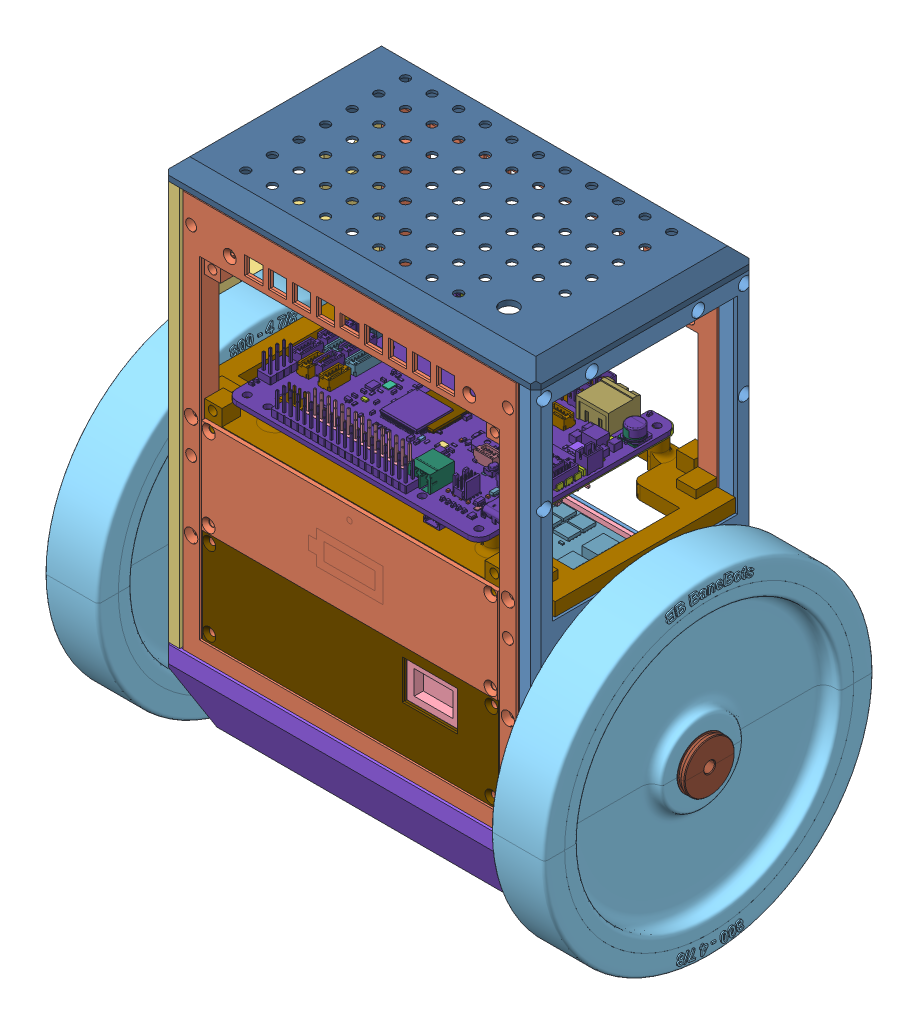
SolidWorks assembly twipr_v2, configuration Default. Lengths in mm.
Overall size (189.01 198.92 123.83).
484 component instances, 75 part files, 68 mates.
Components (placement in the parent):
- twipr_sketch-1: twipr_sketch [Default] at origin size (188 200.75 0) (hidden)
- brace_right-2: brace_right [Default] at (-379.6774 202.2203 0) x (0 0 -1) z (1 0 0) size (82 150 7)
- brace_front_led-1: brace_front_led [Default] at (-442.6774 202.2203 -41) size (126 150 7)
- brace_left_display-2: brace_left_display [Default] at (-505.6774 202.2203 0) x (0 0 1) z (-1 0 0) size (82 150 8)
- brace_front_led-2: brace_front_led [Default] at (-442.6774 202.2203 41) x (-1 0 0) z (0 0 -1) size (126 150 7)
- platform_middle_big_bms-1: platform_middle_big_bms [Default] at (-442.7274 165.7203 0) size (126 42 78.8)
- banebots_4_78-1: banebots_4_78 [Default] at (-368.872 147.2203 0) x (0 0 -1) z (1 0 0) size (123.83 123.83 21.34)
- banebots_4_78-2: banebots_4_78 [Default] at (-516.2261 147.2203 0) x (0 0 1) z (-1 0 0) size (123.83 123.83 21.34)
- robot-hub-1: robot-hub [Default] at (-323.8774 212.8203 108.5) x (-1 0 0) z (0 1 0) size (91.46 70 13.31)
  - robot-hub.step-1: robot-hub.step [Default] at origin size (91.46 70 13.31)
    - R_0603_1608Metric.step-1: R_0603_1608Metric.step [Default] at (112.6 -91.1 1.71) x (0 1 0) z (0 0 1) size (1.6 0.8 0.45)
      - SOLID.step-1: SOLID.step [Default] at origin size (1.6 0.8 0.45)
    - C_1210_3225Metric.step-1: C_1210_3225Metric.step [Default] at (76.55 -102.85 1.71) x (-1 0 0) z (0 0 1) size (3.2 2.5 2.5)
      - SOLID-0.step-1: SOLID-0.step [Default] at origin size (3.2 2.5 2.5)
    - C_0603_1608Metric.step-1: C_0603_1608Metric.step [Default] at (132.2 -95.8 1.71) x (0 1 0) z (0 0 1) size (1.6 0.8 0.8)
      - SOLID-1.step-1: SOLID-1.step [Default] at origin size (1.6 0.8 0.8)
    - JST_GH_BM04B-GHS-TBT_1x04-1MP_P1.25mm_Vertical.step-1: JST_GH_BM04B-GHS-TBT_1x04-1MP_P1.25mm_Vertical.step [Default] at (152.6 -95.3 1.71) x (0 1 0) z (0 0 1) size (8.25 4.95 4.2)
      - SOLID-2.step-1: SOLID-2.step [Default] at origin size (8.25 4.95 4.2)
    - R_0603_1608Metric.step-2: R_0603_1608Metric.step [Default] at (107.5 -84.7687 1.71) x (0 -1 0) z (0 0 1) size (1.6 0.8 0.45)
      - SOLID.step-1: SOLID.step [Default] at origin size (1.6 0.8 0.45)
    - R_0402_1005Metric.step-1: R_0402_1005Metric.step [Default] at (123.5 -93.2 1.71) x (0 1 0) z (0 0 1) size (1 0.5 0.35)
      - SOLID-3.step-1: SOLID-3.step [Default] at origin size (1 0.5 0.35)
    - LED_0603_1608Metric.step-1: LED_0603_1608Metric.step [Default] at (88 -81.3 1.71) x (0 -1 0) z (0 0 1) size (1.6 0.8 1.1)
      - SOLID-4.step-1: SOLID-4.step [Default] at origin size (1.6 0.8 1.1)
    - R_0603_1608Metric.step-3: R_0603_1608Metric.step [Default] at (113.4 -101.6 1.71) x (-1 0 0) z (0 0 1) size (1.6 0.8 0.45)
      - SOLID.step-1: SOLID.step [Default] at origin size (1.6 0.8 0.45)
    - LTC4412ES6#TRMPBF.step-1: LTC4412ES6#TRMPBF.step [Default] at (86.1 -94.6 1.71) size (2.8 2.9 1)
      - COMPOUND.step-1: COMPOUND.step [Default] at origin size (2.8 2.9 1)
    - ws2812_2020.step-1: ws2812_2020.step [Default] at (84.3 -81.3 1.71) size (2.2 2 0.84)
      - COMPOUND-5.step-1: COMPOUND-5.step [Default] at origin size (2.2 2 0.84)
    - LED_0603_1608Metric.step-2: LED_0603_1608Metric.step [Default] at (86.1 -86.8 1.71) size (1.6 0.8 1.1)
      - SOLID-4.step-1: SOLID-4.step [Default] at origin size (1.6 0.8 1.1)
    - R_0402_1005Metric.step-2: R_0402_1005Metric.step [Default] at (133.8 -92.9 1.71) x (0 -1 0) z (0 0 1) size (1 0.5 0.35)
      - SOLID-3.step-1: SOLID-3.step [Default] at origin size (1 0.5 0.35)
    - JST_GH_BM06B-GHS-TBT_1x06-1MP_P1.25mm_Vertical.step-1: JST_GH_BM06B-GHS-TBT_1x06-1MP_P1.25mm_Vertical.step [Default] at (114 -135.2 1.71) size (10.75 4.95 4.2)
      - SOLID-6.step-1: SOLID-6.step [Default] at origin size (10.75 4.95 4.2)
    - JST_GH_BM04B-GHS-TBT_1x04-1MP_P1.25mm_Vertical.step-2: JST_GH_BM04B-GHS-TBT_1x04-1MP_P1.25mm_Vertical.step [Default] at (134.6 -135.2 1.71) size (8.25 4.95 4.2)
      - SOLID-2.step-1: SOLID-2.step [Default] at origin size (8.25 4.95 4.2)
    - C_0603_1608Metric.step-2: C_0603_1608Metric.step [Default] at (109.4 -97.4 1.71) x (-1 0 0) z (0 0 1) size (1.6 0.8 0.8)
      - SOLID-1.step-1: SOLID-1.step [Default] at origin size (1.6 0.8 0.8)
    - C_1210_3225Metric.step-2: C_1210_3225Metric.step [Default] at (87.55 -126.8 1.71) size (3.2 2.5 2.5)
      - SOLID-0.step-1: SOLID-0.step [Default] at origin size (3.2 2.5 2.5)
    - C_1210_3225Metric.step-3: C_1210_3225Metric.step [Default] at (76.55 -109.6 1.71) x (-1 0 0) z (0 0 1) size (3.2 2.5 2.5)
      - SOLID-0.step-1: SOLID-0.step [Default] at origin size (3.2 2.5 2.5)
    - R_0603_1608Metric.step-4: R_0603_1608Metric.step [Default] at (138.6 -95.5 1.71) x (0 -1 0) z (0 0 1) size (1.6 0.8 0.45)
      - SOLID.step-1: SOLID.step [Default] at origin size (1.6 0.8 0.45)
    - CP_Elec_6.3x5.2.step-1: CP_Elec_6.3x5.2.step [Default] at (77.8 -133.7 1.71) x (0 1 0) z (0 0 1) size (10.2 10.92 5.2)
      - SOLID-7.step-1: SOLID-7.step [Default] at origin size (10.2 10.92 5.2)
    - R_0402_1005Metric.step-3: R_0402_1005Metric.step [Default] at (127.9 -91.7 1.71) x (0 -1 0) z (0 0 1) size (1 0.5 0.35)
      - SOLID-3.step-1: SOLID-3.step [Default] at origin size (1 0.5 0.35)
    - R_0603_1608Metric.step-5: R_0603_1608Metric.step [Default] at (104.2 -119.8 1.71) size (1.6 0.8 0.45)
      - SOLID.step-1: SOLID.step [Default] at origin size (1.6 0.8 0.45)
    - C_0603_1608Metric.step-3: C_0603_1608Metric.step [Default] at (132 -113.2 1.71) x (0 -1 0) z (0 0 1) size (1.6 0.8 0.8)
      - SOLID-1.step-1: SOLID-1.step [Default] at origin size (1.6 0.8 0.8)
    - JST_GH_BM04B-GHS-TBT_1x04-1MP_P1.25mm_Vertical.step-3: JST_GH_BM04B-GHS-TBT_1x04-1MP_P1.25mm_Vertical.step [Default] at (97.4 -125.1 1.71) size (8.25 4.95 4.2)
      - SOLID-2.step-1: SOLID-2.step [Default] at origin size (8.25 4.95 4.2)
    - C_0603_1608Metric.step-4: C_0603_1608Metric.step [Default] at (87.8 -117.65 1.71) x (0 -1 0) z (0 0 1) size (1.6 0.8 0.8)
      - SOLID-1.step-1: SOLID-1.step [Default] at origin size (1.6 0.8 0.8)
    - JST_GH_BM06B-GHS-TBT_1x06-1MP_P1.25mm_Vertical.step-2: JST_GH_BM06B-GHS-TBT_1x06-1MP_P1.25mm_Vertical.step [Default] at (160.6 -106.3 1.71) x (0 1 0) z (0 0 1) size (10.75 4.95 4.2)
      - SOLID-6.step-1: SOLID-6.step [Default] at origin size (10.75 4.95 4.2)
    - JST_GH_BM02B-GHS-TBT_1x02-1MP_P1.25mm_Vertical.step-1: JST_GH_BM02B-GHS-TBT_1x02-1MP_P1.25mm_Vertical.step [Default] at (152.5 -143.25 1.71) size (5.75 4.95 4.2)
      - SOLID-8.step-1: SOLID-8.step [Default] at origin size (5.75 4.95 4.2)
    - USB4105-GF-A.step-1: USB4105-GF-A.step [Default] at (76.635 -88.9375 1.71) x (0 -1 0) z (-1 0 0) size (9.58 4.16 7.71)
      - COMPOUND-9.step-1: COMPOUND-9.step [Default] at origin size (9.58 4.16 7.71)
    - JST_GH_BM04B-GHS-TBT_1x04-1MP_P1.25mm_Vertical.step-4: JST_GH_BM04B-GHS-TBT_1x04-1MP_P1.25mm_Vertical.step [Default] at (160.6 -95.3 1.71) x (0 1 0) z (0 0 1) size (8.25 4.95 4.2)
      - SOLID-2.step-1: SOLID-2.step [Default] at origin size (8.25 4.95 4.2)
    - 4341x30258x6 (rev1).step-1: 4341x30258x6 (rev1).step [Default] at (104.2 -116 1.71) x (1 0 0) z (0 -1 0) size (3.2 2.5 4.6)
      - COMPOUND-10.step-1: COMPOUND-10.step [Default] at origin size (3.2 2.5 4.6)
    - JST_GH_BM04B-GHS-TBT_1x04-1MP_P1.25mm_Vertical.step-5: JST_GH_BM04B-GHS-TBT_1x04-1MP_P1.25mm_Vertical.step [Default] at (103.2 -143.2 1.71) size (8.25 4.95 4.2)
      - SOLID-2.step-1: SOLID-2.step [Default] at origin size (8.25 4.95 4.2)
    - C_0805_2012Metric.step-1: C_0805_2012Metric.step [Default] at (112.7 -112 1.71) x (0 1 0) z (0 0 1) size (2 1.25 1.25)
      - SOLID-11.step-1: SOLID-11.step [Default] at origin size (2 1.25 1.25)
    - CUI_DEVICES_CMT-7525-80-SMT-TR.step-1: CUI_DEVICES_CMT-7525-80-SMT-TR.step [Default] at (97.3 -115.8 1.71) x (1 0 0) z (0 -1 0) size (7.5 2.5 7.5)
      - COMPOUND-12.step-1: COMPOUND-12.step [Default] at origin size (7.5 2.5 7.5)
    - BMX160.step-1: BMX160.step [Default] at (111.35 -94.75 1.71) x (0 -1 0) z (-1 0 0) size (3 1 2.5)
      - COMPOUND-13.step-1: COMPOUND-13.step [Default] at origin size (3 1 2.5)
    - PinHeader_2x15_P2.54mm_Vertical.step-1: PinHeader_2x15_P2.54mm_Vertical.step [Default] at (110.525 -127.545 1.71) x (0 1 0) z (0 0 1) size (5.08 38.1 11.54)
      - SOLID-14.step-1: SOLID-14.step [Default] at origin size (5.08 38.1 11.54)
    - C_0603_1608Metric.step-5: C_0603_1608Metric.step [Default] at (115.5 -93.3 1.71) x (0 1 0) z (0 0 1) size (1.6 0.8 0.8)
      - SOLID-1.step-1: SOLID-1.step [Default] at origin size (1.6 0.8 0.8)
    - JST_GH_BM02B-GHS-TBT_1x02-1MP_P1.25mm_Vertical.step-2: JST_GH_BM02B-GHS-TBT_1x02-1MP_P1.25mm_Vertical.step [Default] at (152.5 -135.25 1.71) size (5.75 4.95 4.2)
      - SOLID-8.step-1: SOLID-8.step [Default] at origin size (5.75 4.95 4.2)
    - FTSH-105-01-L-DV-K.step-1: FTSH-105-01-L-DV-K.step [Default] at (97.4 -106.5 2.21) x (-1 0 0) z (0 1 0) size (6.35 6.12 5.84)
      - COMPOUND-15.step-1: COMPOUND-15.step [Default] at origin size (6.35 6.12 5.84)
    - JST_GH_BM04B-GHS-TBT_1x04-1MP_P1.25mm_Vertical.step-6: JST_GH_BM04B-GHS-TBT_1x04-1MP_P1.25mm_Vertical.step [Default] at (103.2 -135.2 1.71) size (8.25 4.95 4.2)
      - SOLID-2.step-1: SOLID-2.step [Default] at origin size (8.25 4.95 4.2)
    - C_0603_1608Metric.step-6: C_0603_1608Metric.step [Default] at (141.5 -98.8 1.71) x (0 1 0) z (0 0 1) size (1.6 0.8 0.8)
      - SOLID-1.step-1: SOLID-1.step [Default] at origin size (1.6 0.8 0.8)
    - ECS-250-18-33B-CKY-TR.step-1: ECS-250-18-33B-CKY-TR.step [Default] at (140.9 -104.6 1.71) x (0 1 0) z (0 0 1) size (3.38 2.78 0.9)
      - COMPOUND-16.step-1: COMPOUND-16.step [Default] at origin size (3.38 2.78 0.9)
    - C_0603_1608Metric.step-7: C_0603_1608Metric.step [Default] at (114.5 -112.3 1.71) x (0 1 0) z (0 0 1) size (1.6 0.8 0.8)
      - SOLID-1.step-1: SOLID-1.step [Default] at origin size (1.6 0.8 0.8)
    - JST_GH_BM06B-GHS-TBT_1x06-1MP_P1.25mm_Vertical.step-3: JST_GH_BM06B-GHS-TBT_1x06-1MP_P1.25mm_Vertical.step [Default] at (113.95 -143.2 1.71) size (10.75 4.95 4.2)
      - SOLID-6.step-1: SOLID-6.step [Default] at origin size (10.75 4.95 4.2)
    - C_0603_1608Metric.step-8: C_0603_1608Metric.step [Default] at (134.9 -106.6 1.71) x (0 -1 0) z (0 0 1) size (1.6 0.8 0.8)
      - SOLID-1.step-1: SOLID-1.step [Default] at origin size (1.6 0.8 0.8)
    - SOT-323_SC-70.step-1: SOT-323_SC-70.step [Default] at (140.9 -95.4 1.71) x (0 1 0) z (0 0 1) size (2 2 1.05)
      - SOLID-17.step-1: SOLID-17.step [Default] at origin size (2 2 1.05)
    - LED_0603_1608Metric.step-3: LED_0603_1608Metric.step [Default] at (109.4 -100.1 1.71) x (0 -1 0) z (0 0 1) size (1.6 0.8 1.1)
      - SOLID-4.step-1: SOLID-4.step [Default] at origin size (1.6 0.8 1.1)
    - LMR33630ADDA.step-1: LMR33630ADDA.step [Default] at (84.05 -119.1 1.71) x (0 1 0) z (0 0 1) size (6 4.9 1.7)
      - COMPOUND-18.step-1: COMPOUND-18.step [Default] at origin size (6 4.9 1.7)
    - C_0603_1608Metric.step-9: C_0603_1608Metric.step [Default] at (88.3 -124.4 1.71) size (1.6 0.8 0.8)
      - SOLID-1.step-1: SOLID-1.step [Default] at origin size (1.6 0.8 0.8)
    - C_0603_1608Metric.step-10: C_0603_1608Metric.step [Default] at (140.8 -101.1 1.71) size (1.6 0.8 0.8)
      - SOLID-1.step-1: SOLID-1.step [Default] at origin size (1.6 0.8 0.8)
    - PinHeader_2x04_P2.00mm_Vertical.step-1: PinHeader_2x04_P2.00mm_Vertical.step [Default] at (149.4 -81.4 1.71) x (0 1 0) z (0 0 1) size (4 8 8.8)
      - SOLID-19.step-1: SOLID-19.step [Default] at origin size (4 8 8.8)
    - 1-1734248-5.step-1: 1-1734248-5.step [Default] at (159.98 -126.3 6.21) x (0 1 0) z (0 0 1) size (22.4 4.85 5.68)
      - SOLID-20.step-1: SOLID-20.step [Default] at origin size (22.4 4.85 5.68)
    - IS25LP032D-JNLA3-TR.step-1: IS25LP032D-JNLA3-TR.step [Default] at (84.9 -99.3 1.71) x (-1 0 0) z (0 0 1) size (6 4.9 1.75)
      - COMPOUND-21.step-1: COMPOUND-21.step [Default] at origin size (6 4.9 1.75)
    - 691313510002.step-1: 691313510002.step [Default] at (89.3 -135.2 5.71) x (-1 0 0) z (0 -1 0) size (12.16 12 12)
      - COMPOUND-22.step-1: COMPOUND-22.step [Default] at origin size (12.16 12 12)
    - LED_0603_1608Metric.step-4: LED_0603_1608Metric.step [Default] at (93 -81.3 1.71) x (0 -1 0) z (0 0 1) size (1.6 0.8 1.1)
      - SOLID-4.step-1: SOLID-4.step [Default] at origin size (1.6 0.8 1.1)
    - JST_GH_BM04B-GHS-TBT_1x04-1MP_P1.25mm_Vertical.step-7: JST_GH_BM04B-GHS-TBT_1x04-1MP_P1.25mm_Vertical.step [Default] at (124.95 -135.2 1.71) size (8.25 4.95 4.2)
      - SOLID-2.step-1: SOLID-2.step [Default] at origin size (8.25 4.95 4.2)
    - LED_0603_1608Metric.step-5: LED_0603_1608Metric.step [Default] at (154.5 -117.4 1.71) x (0 -1 0) z (0 0 1) size (1.6 0.8 1.1)
      - SOLID-4.step-1: SOLID-4.step [Default] at origin size (1.6 0.8 1.1)
    - JST_GH_BM03B-GHS-TBT_1x03-1MP_P1.25mm_Vertical.step-1: JST_GH_BM03B-GHS-TBT_1x03-1MP_P1.25mm_Vertical.step [Default] at (97.4 -98.7 1.71) size (7 4.95 4.2)
      - SOLID-23.step-1: SOLID-23.step [Default] at origin size (7 4.95 4.2)
    - C_0603_1608Metric.step-11: C_0603_1608Metric.step [Default] at (108.6 -94.8 1.71) x (0 -1 0) z (0 0 1) size (1.6 0.8 0.8)
      - SOLID-1.step-1: SOLID-1.step [Default] at origin size (1.6 0.8 0.8)
    - R_0603_1608Metric.step-6: R_0603_1608Metric.step [Default] at (113.4 -103.2 1.71) size (1.6 0.8 0.45)
      - SOLID.step-1: SOLID.step [Default] at origin size (1.6 0.8 0.45)
    - LED_0603_1608Metric.step-6: LED_0603_1608Metric.step [Default] at (95.5 -81.3 1.71) x (0 -1 0) z (0 0 1) size (1.6 0.8 1.1)
      - SOLID-4.step-1: SOLID-4.step [Default] at origin size (1.6 0.8 1.1)
    - R_0402_1005Metric.step-4: R_0402_1005Metric.step [Default] at (125.7 -93.2 1.71) x (0 -1 0) z (0 0 1) size (1 0.5 0.35)
      - SOLID-3.step-1: SOLID-3.step [Default] at origin size (1 0.5 0.35)
    - SOT-23-6.step-1: SOT-23-6.step [Default] at (86.1 -89.45 1.71) x (-1 0 0) z (0 0 1) size (2.8 2.9 1.55)
      - SOLID-24.step-1: SOLID-24.step [Default] at origin size (2.8 2.9 1.55)
    - R_0603_1608Metric.step-7: R_0603_1608Metric.step [Default] at (89.3 -117.65 1.71) x (0 -1 0) z (0 0 1) size (1.6 0.8 0.45)
      - SOLID.step-1: SOLID.step [Default] at origin size (1.6 0.8 0.45)
    - R_0603_1608Metric.step-8: R_0603_1608Metric.step [Default] at (92.3 -111.9 1.71) x (0 1 0) z (0 0 1) size (1.6 0.8 0.45)
      - SOLID.step-1: SOLID.step [Default] at origin size (1.6 0.8 0.45)
    - R_0603_1608Metric.step-9: R_0603_1608Metric.step [Default] at (88.55 -115.4 1.71) size (1.6 0.8 0.45)
      - SOLID.step-1: SOLID.step [Default] at origin size (1.6 0.8 0.45)
    - 691322110002.step-1: 691322110002.step [Default] at (101.9 -81.4 5.21) x (-1 0 0) z (0 1 0) size (8.4 10.7 9.2)
      - COMPOUND-25.step-1: COMPOUND-25.step [Default] at origin size (8.4 10.7 9.2)
    - LED_0603_1608Metric.step-7: LED_0603_1608Metric.step [Default] at (90.5 -81.3 1.71) x (0 -1 0) z (0 0 1) size (1.6 0.8 1.1)
      - SOLID-4.step-1: SOLID-4.step [Default] at origin size (1.6 0.8 1.1)
    - JST_GH_BM06B-GHS-TBT_1x06-1MP_P1.25mm_Vertical.step-4: JST_GH_BM06B-GHS-TBT_1x06-1MP_P1.25mm_Vertical.step [Default] at (152.6 -106.3 1.71) x (0 1 0) z (0 0 1) size (10.75 4.95 4.2)
      - SOLID-6.step-1: SOLID-6.step [Default] at origin size (10.75 4.95 4.2)
    - R_0603_1608Metric.step-10: R_0603_1608Metric.step [Default] at (140 -98.8 1.71) x (0 -1 0) z (0 0 1) size (1.6 0.8 0.45)
      - SOLID.step-1: SOLID.step [Default] at origin size (1.6 0.8 0.45)
    - C_1210_3225Metric.step-4: C_1210_3225Metric.step [Default] at (79.6 -126.9 1.71) x (-1 0 0) z (0 0 1) size (3.2 2.5 2.5)
      - SOLID-0.step-1: SOLID-0.step [Default] at origin size (3.2 2.5 2.5)
    - JST_GH_BM04B-GHS-TBT_1x04-1MP_P1.25mm_Vertical.step-8: JST_GH_BM04B-GHS-TBT_1x04-1MP_P1.25mm_Vertical.step [Default] at (134.6 -143.2 1.71) size (8.25 4.95 4.2)
      - SOLID-2.step-1: SOLID-2.step [Default] at origin size (8.25 4.95 4.2)
    - PDS760-13.step-1: PDS760-13.step [Default] at (77.99 -118.49 1.71) x (1 0 0) z (0 -1 0) size (3.9 1.05 6.4)
      - COMPOUND-26.step-1: COMPOUND-26.step [Default] at origin size (3.9 1.05 6.4)
    - PinHeader_2x15_P2.54mm_Vertical.step-2: PinHeader_2x15_P2.54mm_Vertical.step [Default] at (110.525 -81.825 1.71) x (0 1 0) z (0 0 1) size (5.08 38.1 11.54)
      - SOLID-14.step-1: SOLID-14.step [Default] at origin size (5.08 38.1 11.54)
    - LED_0603_1608Metric.step-8: LED_0603_1608Metric.step [Default] at (96.8 -143.9 1.71) x (0 -1 0) z (0 0 1) size (1.6 0.8 1.1)
      - SOLID-4.step-1: SOLID-4.step [Default] at origin size (1.6 0.8 1.1)
    - 744325.step-1: 744325.step [Default] at (84.55 -108.35 1.71) x (-1 0 0) z (0 0 1) size (10.74 11.01 5.01)
      - COMPOUND-27.step-1: COMPOUND-27.step [Default] at origin size (10.74 11.01 5.01)
    - R_0603_1608Metric.step-11: R_0603_1608Metric.step [Default] at (111.05 -91.05 1.71) x (0 1 0) z (0 0 1) size (1.6 0.8 0.45)
      - SOLID.step-1: SOLID.step [Default] at origin size (1.6 0.8 0.45)
    - C_0603_1608Metric.step-12: C_0603_1608Metric.step [Default] at (140.75 -108.7 1.71) x (-1 0 0) z (0 0 1) size (1.6 0.8 0.8)
      - SOLID-1.step-1: SOLID-1.step [Default] at origin size (1.6 0.8 0.8)
    - C_0603_1608Metric.step-13: C_0603_1608Metric.step [Default] at (135.6 -109.2 1.71) size (1.6 0.8 0.8)
      - SOLID-1.step-1: SOLID-1.step [Default] at origin size (1.6 0.8 0.8)
    - R_0603_1608Metric.step-12: R_0603_1608Metric.step [Default] at (140.7 -111 1.71) size (1.6 0.8 0.45)
      - SOLID.step-1: SOLID.step [Default] at origin size (1.6 0.8 0.45)
    - LQFP-100_14x14mm_P0.5mm.step-1: LQFP-100_14x14mm_P0.5mm.step [Default] at (124 -104.2 1.71) x (-1 0 0) z (0 0 1) size (16 16 1.5)
      - SOLID-28.step-1: SOLID-28.step [Default] at origin size (16 16 1.5)
    - R_0603_1608Metric.step-13: R_0603_1608Metric.step [Default] at (87.8 -120.65 1.71) x (0 1 0) z (0 0 1) size (1.6 0.8 0.45)
      - SOLID.step-1: SOLID.step [Default] at origin size (1.6 0.8 0.45)
    - C_1210_3225Metric.step-5: C_1210_3225Metric.step [Default] at (76.55 -112.85 1.71) x (-1 0 0) z (0 0 1) size (3.2 2.5 2.5)
      - SOLID-0.step-1: SOLID-0.step [Default] at origin size (3.2 2.5 2.5)
    - R_0402_1005Metric.step-5: R_0402_1005Metric.step [Default] at (124.6 -93.2 1.71) x (0 1 0) z (0 0 1) size (1 0.5 0.35)
      - SOLID-3.step-1: SOLID-3.step [Default] at origin size (1 0.5 0.35)
    - SOT-563.step-1: SOT-563.step [Default] at (94.4 -93.9 1.71) x (0 -1 0) z (0 0 1) size (1.6 1.6 0.63)
      - SOLID-29.step-1: SOLID-29.step [Default] at origin size (1.6 1.6 0.63)
    - JST_GH_BM04B-GHS-TBT_1x04-1MP_P1.25mm_Vertical.step-9: JST_GH_BM04B-GHS-TBT_1x04-1MP_P1.25mm_Vertical.step [Default] at (144.225 -143.2344 1.71) size (8.25 4.95 4.2)
      - SOLID-2.step-1: SOLID-2.step [Default] at origin size (8.25 4.95 4.2)
    - C_1210_3225Metric.step-6: C_1210_3225Metric.step [Default] at (76.55 -106.35 1.71) x (-1 0 0) z (0 0 1) size (3.2 2.5 2.5)
      - SOLID-0.step-1: SOLID-0.step [Default] at origin size (3.2 2.5 2.5)
    - C_0603_1608Metric.step-14: C_0603_1608Metric.step [Default] at (79.8 -123.6 1.71) x (-1 0 0) z (0 0 1) size (1.6 0.8 0.8)
      - SOLID-1.step-1: SOLID-1.step [Default] at origin size (1.6 0.8 0.8)
    - R_0402_1005Metric.step-6: R_0402_1005Metric.step [Default] at (129 -91.7 1.71) x (0 -1 0) z (0 0 1) size (1 0.5 0.35)
      - SOLID-3.step-1: SOLID-3.step [Default] at origin size (1 0.5 0.35)
    - LED_0603_1608Metric.step-9: LED_0603_1608Metric.step [Default] at (107.5 -81.6688 1.71) x (0 -1 0) z (0 0 1) size (1.6 0.8 1.1)
      - SOLID-4.step-1: SOLID-4.step [Default] at origin size (1.6 0.8 1.1)
    - JST_GH_BM04B-GHS-TBT_1x04-1MP_P1.25mm_Vertical.step-10: JST_GH_BM04B-GHS-TBT_1x04-1MP_P1.25mm_Vertical.step [Default] at (124.95 -143.2 1.71) size (8.25 4.95 4.2)
      - SOLID-2.step-1: SOLID-2.step [Default] at origin size (8.25 4.95 4.2)
    - LED_0603_1608Metric.step-10: LED_0603_1608Metric.step [Default] at (152.6 -117.4 1.71) x (0 -1 0) z (0 0 1) size (1.6 0.8 1.1)
      - SOLID-4.step-1: SOLID-4.step [Default] at origin size (1.6 0.8 1.1)
    - C_0805_2012Metric.step-2: C_0805_2012Metric.step [Default] at (117.4 -93.1 1.71) x (0 -1 0) z (0 0 1) size (2 1.25 1.25)
      - SOLID-11.step-1: SOLID-11.step [Default] at origin size (2 1.25 1.25)
    - C_0603_1608Metric.step-15: C_0603_1608Metric.step [Default] at (135 -100.5 1.71) x (0 -1 0) z (0 0 1) size (1.6 0.8 0.8)
      - SOLID-1.step-1: SOLID-1.step [Default] at origin size (1.6 0.8 0.8)
    - R_0603_1608Metric.step-14: R_0603_1608Metric.step [Default] at (89 -94.6 1.71) x (0 -1 0) z (0 0 1) size (1.6 0.8 0.45)
      - SOLID.step-1: SOLID.step [Default] at origin size (1.6 0.8 0.45)
    - JST_GH_BM04B-GHS-TBT_1x04-1MP_P1.25mm_Vertical.step-11: JST_GH_BM04B-GHS-TBT_1x04-1MP_P1.25mm_Vertical.step [Default] at (144.225 -135.2344 1.71) size (8.25 4.95 4.2)
      - SOLID-2.step-1: SOLID-2.step [Default] at origin size (8.25 4.95 4.2)
    - R_0603_1608Metric.step-15: R_0603_1608Metric.step [Default] at (99.6 -129.6 -0.05) x (0 1 0) z (0 0 -1) size (1.6 0.8 0.45)
      - SOLID.step-1: SOLID.step [Default] at origin size (1.6 0.8 0.45)
    - C_0603_1608Metric.step-16: C_0603_1608Metric.step [Default] at (131.9625 -133.35 -0.05) x (0 1 0) z (0 0 -1) size (1.6 0.8 0.8)
      - SOLID-1.step-1: SOLID-1.step [Default] at origin size (1.6 0.8 0.8)
    - R_0603_1608Metric.step-16: R_0603_1608Metric.step [Default] at (119.6 -120.9 -0.05) x (-1 0 0) z (0 0 -1) size (1.6 0.8 0.45)
      - SOLID.step-1: SOLID.step [Default] at origin size (1.6 0.8 0.45)
    - R_0402_1005Metric.step-7: R_0402_1005Metric.step [Default] at (97.7 -85.3 -0.05) x (0 1 0) z (0 0 -1) size (1 0.5 0.35)
      - SOLID-3.step-1: SOLID-3.step [Default] at origin size (1 0.5 0.35)
    - C_0805_2012Metric.step-3: C_0805_2012Metric.step [Default] at (92.5 -98.9 -0.05) x (0 -1 0) z (0 0 -1) size (2 1.25 1.25)
      - SOLID-11.step-1: SOLID-11.step [Default] at origin size (2 1.25 1.25)
    - R_0402_1005Metric.step-8: R_0402_1005Metric.step [Default] at (91.95 -90.35 -0.05) x (-1 0 0) z (0 0 -1) size (1 0.5 0.35)
      - SOLID-3.step-1: SOLID-3.step [Default] at origin size (1 0.5 0.35)
    - MSOP-10_3x3mm_P0.5mm.step-1: MSOP-10_3x3mm_P0.5mm.step [Default] at (111.8 -114.8 -0.05) x (-1 0 0) z (0 0 -1) size (4.9 3 0.95)
      - SOLID-30.step-1: SOLID-30.step [Default] at origin size (4.9 3 0.95)
    - STM32G031G6U6.step-1: STM32G031G6U6.step [Default] at (95.6 -89.05 -0.05) x (0 1 0) z (0 0 -1) size (4.1 4.1 0.6)
      - COMPOUND-31.step-1: COMPOUND-31.step [Default] at origin size (4.1 4.1 0.6)
    - R_0603_1608Metric.step-17: R_0603_1608Metric.step [Default] at (137.5 -144 -0.05) x (0 -1 0) z (0 0 -1) size (1.6 0.8 0.45)
      - SOLID.step-1: SOLID.step [Default] at origin size (1.6 0.8 0.45)
    - R_0603_1608Metric.step-18: R_0603_1608Metric.step [Default] at (137.4625 -136.35 -0.05) x (0 -1 0) z (0 0 -1) size (1.6 0.8 0.45)
      - SOLID.step-1: SOLID.step [Default] at origin size (1.6 0.8 0.45)
    - C_0603_1608Metric.step-17: C_0603_1608Metric.step [Default] at (139 -140.9 -0.05) x (0 1 0) z (0 0 -1) size (1.6 0.8 0.8)
      - SOLID-1.step-1: SOLID-1.step [Default] at origin size (1.6 0.8 0.8)
    - R_0603_1608Metric.step-19: R_0603_1608Metric.step [Default] at (97.5 -137.2 -0.05) x (0 1 0) z (0 0 -1) size (1.6 0.8 0.45)
      - SOLID.step-1: SOLID.step [Default] at origin size (1.6 0.8 0.45)
    - R_0603_1608Metric.step-20: R_0603_1608Metric.step [Default] at (117.6 -113.8 -0.05) x (-1 0 0) z (0 0 -1) size (1.6 0.8 0.45)
      - SOLID.step-1: SOLID.step [Default] at origin size (1.6 0.8 0.45)
    - R_0603_1608Metric.step-21: R_0603_1608Metric.step [Default] at (156.7 -115 -0.05) x (0 1 0) z (0 0 -1) size (1.6 0.8 0.45)
      - SOLID.step-1: SOLID.step [Default] at origin size (1.6 0.8 0.45)
    - C_0603_1608Metric.step-18: C_0603_1608Metric.step [Default] at (126.85 -136.2 -0.05) x (0 1 0) z (0 0 -1) size (1.6 0.8 0.8)
      - SOLID-1.step-1: SOLID-1.step [Default] at origin size (1.6 0.8 0.8)
    - R_0603_1608Metric.step-22: R_0603_1608Metric.step [Default] at (97.9 -129.6 -0.05) x (0 1 0) z (0 0 -1) size (1.6 0.8 0.45)
      - SOLID.step-1: SOLID.step [Default] at origin size (1.6 0.8 0.45)
    - C_0805_2012Metric.step-4: C_0805_2012Metric.step [Default] at (99.15 -100.9 -0.05) x (0 1 0) z (0 0 -1) size (2 1.25 1.25)
      - SOLID-11.step-1: SOLID-11.step [Default] at origin size (2 1.25 1.25)
    - R_0402_1005Metric.step-9: R_0402_1005Metric.step [Default] at (88.15 -88.95 -0.05) x (0 -1 0) z (0 0 -1) size (1 0.5 0.35)
      - SOLID-3.step-1: SOLID-3.step [Default] at origin size (1 0.5 0.35)
    - R_0603_1608Metric.step-23: R_0603_1608Metric.step [Default] at (96.3 -129.6 -0.05) x (0 1 0) z (0 0 -1) size (1.6 0.8 0.45)
      - SOLID.step-1: SOLID.step [Default] at origin size (1.6 0.8 0.45)
    - R_0402_1005Metric.step-10: R_0402_1005Metric.step [Default] at (91.96 -86.35 -0.05) x (-1 0 0) z (0 0 -1) size (1 0.5 0.35)
      - SOLID-3.step-1: SOLID-3.step [Default] at origin size (1 0.5 0.35)
    - Fuse_1206_3216Metric.step-1: Fuse_1206_3216Metric.step [Default] at (82.7 -138.7 -0.05) x (-1 0 0) z (0 0 -1) size (3.2 1.6 0.55)
      - SOLID-32.step-1: SOLID-32.step [Default] at origin size (3.2 1.6 0.55)
    - R_0603_1608Metric.step-24: R_0603_1608Metric.step [Default] at (125.4 -130.4 -0.05) x (0 -1 0) z (0 0 -1) size (1.6 0.8 0.45)
      - SOLID.step-1: SOLID.step [Default] at origin size (1.6 0.8 0.45)
    - R_0603_1608Metric.step-25: R_0603_1608Metric.step [Default] at (144.7 -142.2 -0.05) x (1 0 0) z (0 0 -1) size (1.6 0.8 0.45)
      - SOLID.step-1: SOLID.step [Default] at origin size (1.6 0.8 0.45)
    - R_0603_1608Metric.step-26: R_0603_1608Metric.step [Default] at (151.2 -84.3 -0.05) x (0 1 0) z (0 0 -1) size (1.6 0.8 0.45)
      - SOLID.step-1: SOLID.step [Default] at origin size (1.6 0.8 0.45)
    - R_0603_1608Metric.step-27: R_0603_1608Metric.step [Default] at (96 -137.2 -0.05) x (0 1 0) z (0 0 -1) size (1.6 0.8 0.45)
      - SOLID.step-1: SOLID.step [Default] at origin size (1.6 0.8 0.45)
    - R_0603_1608Metric.step-28: R_0603_1608Metric.step [Default] at (104.5 -106.1 -0.05) x (-1 0 0) z (0 0 -1) size (1.6 0.8 0.45)
      - SOLID.step-1: SOLID.step [Default] at origin size (1.6 0.8 0.45)
    - DF40C-100DS.step-1: DF40C-100DS.step [Default] at (144.62 -86.64 -0.05) x (0 -1 0) z (1 0 0) size (3.38 1.45 22.6)
      - SOLID-33.step-1: SOLID-33.step [Default] at origin size (3.38 1.45 22.6)
    - DF40C-100DS.step-2: DF40C-100DS.step [Default] at (144.62 -120.56 -0.05) x (0 -1 0) z (1 0 0) size (3.38 1.45 22.6)
      - SOLID-33.step-1: SOLID-33.step [Default] at origin size (3.38 1.45 22.6)
    - R_0603_1608Metric.step-29: R_0603_1608Metric.step [Default] at (96.8 -143.9 -0.05) x (0 -1 0) z (0 0 -1) size (1.6 0.8 0.45)
      - SOLID.step-1: SOLID.step [Default] at origin size (1.6 0.8 0.45)
    - C_0603_1608Metric.step-19: C_0603_1608Metric.step [Default] at (137.4625 -133.3 -0.05) x (0 1 0) z (0 0 -1) size (1.6 0.8 0.8)
      - SOLID-1.step-1: SOLID-1.step [Default] at origin size (1.6 0.8 0.8)
    - R_0603_1608Metric.step-30: R_0603_1608Metric.step [Default] at (92.9 -93.2 -0.05) x (0 -1 0) z (0 0 -1) size (1.6 0.8 0.45)
      - SOLID.step-1: SOLID.step [Default] at origin size (1.6 0.8 0.45)
    - C_0805_2012Metric.step-5: C_0805_2012Metric.step [Default] at (101.6 -119.9 -0.05) x (0 -1 0) z (0 0 -1) size (2 1.25 1.25)
      - SOLID-11.step-1: SOLID-11.step [Default] at origin size (2 1.25 1.25)
    - MC74VHC1G14DTT1G.step-1: MC74VHC1G14DTT1G.step [Default] at (157.4 -110.9 -0.05) x (0 -1 0) z (0 0 -1) size (2.75 3 1.1)
      - COMPOUND-34.step-1: COMPOUND-34.step [Default] at origin size (2.75 3 1.1)
    - R_0603_1608Metric.step-31: R_0603_1608Metric.step [Default] at (158.3 -115 -0.05) x (0 1 0) z (0 0 -1) size (1.6 0.8 0.45)
      - SOLID.step-1: SOLID.step [Default] at origin size (1.6 0.8 0.45)
    - C_0603_1608Metric.step-20: C_0603_1608Metric.step [Default] at (88.4 -93.2 -0.05) x (0 -1 0) z (0 0 -1) size (1.6 0.8 0.8)
      - SOLID-1.step-1: SOLID-1.step [Default] at origin size (1.6 0.8 0.8)
    - 9774030151 (rev1).step-1: 9774030151 (rev1).step [Default] at (160 -87.1 -0.05) x (-1 0 0) z (0 0 -1) size (5.1 5.89 4.4)
      - SOLID-35.step-1: SOLID-35.step [Default] at origin size (5.1 5.89 4.4)
    - D_SOD-323F.step-1: D_SOD-323F.step [Default] at (96.1 -113.45 -0.05) x (-1 0 0) z (0 0 -1) size (2.5 1.25 0.73)
      - SOLID-36.step-1: SOLID-36.step [Default] at origin size (2.5 1.25 0.73)
    - SM04B-SRSS-TB_dark.step-1: SM04B-SRSS-TB_dark.step [Default] at (86.2 -81 0.2) x (1 0 0) z (0 1 0) size (6 2.96 4.95)
      - SOLID-37.step-1: SOLID-37.step [Default] at origin size (6 2.96 4.95)
    - 9774030151 (rev1).step-2: 9774030151 (rev1).step [Default] at (112 -120.1 -0.05) x (-1 0 0) z (0 0 -1) size (5.1 5.89 4.4)
      - SOLID-35.step-1: SOLID-35.step [Default] at origin size (5.1 5.89 4.4)
    - M24512-DFDW6TP.step-1: M24512-DFDW6TP.step [Default] at (121.95 -135.9 -0.05) x (1 0 0) z (0 0 -1) size (6.4 3 1.2)
      - COMPOUND-38.step-1: COMPOUND-38.step [Default] at origin size (6.4 3 1.2)
    - C_0603_1608Metric.step-21: C_0603_1608Metric.step [Default] at (126.8 -141.9 -0.05) x (0 1 0) z (0 0 -1) size (1.6 0.8 0.8)
      - SOLID-1.step-1: SOLID-1.step [Default] at origin size (1.6 0.8 0.8)
    - IRF7319TRPBF.step-1: IRF7319TRPBF.step [Default] at (152.8 -137.5 -0.05) x (0 -1 0) z (0 0 -1) size (6 4.9 1.75)
      - COMPOUND-39.step-1: COMPOUND-39.step [Default] at origin size (6 4.9 1.75)
    - SX1508BIULTRT.step-1: SX1508BIULTRT.step [Default] at (120.1 -86 -0.05) x (-1 0 0) z (0 0 -1) size (3.1 3.1 0.6)
      - COMPOUND-40.step-1: COMPOUND-40.step [Default] at origin size (3.1 3.1 0.6)
    - R_0603_1608Metric.step-32: R_0603_1608Metric.step [Default] at (147.2 -130.6 -0.05) x (0 1 0) z (0 0 -1) size (1.6 0.8 0.45)
      - SOLID.step-1: SOLID.step [Default] at origin size (1.6 0.8 0.45)
    - LTC4365CTS8#TRMPBF.step-1: LTC4365CTS8#TRMPBF.step [Default] at (91.3 -135.6 -0.05) x (-1 0 0) z (0 0 -1) size (2.8 2.9 1)
      - COMPOUND-41.step-1: COMPOUND-41.step [Default] at origin size (2.8 2.9 1)
    - C_0603_1608Metric.step-22: C_0603_1608Metric.step [Default] at (106.5 -133.3 -0.05) x (0 -1 0) z (0 0 -1) size (1.6 0.8 0.8)
      - SOLID-1.step-1: SOLID-1.step [Default] at origin size (1.6 0.8 0.8)
    - SOT-323_SC-70.step-2: SOT-323_SC-70.step [Default] at (92.8 -112.95 -0.05) x (0 -1 0) z (0 0 -1) size (2 2 1.05)
      - SOLID-17.step-1: SOLID-17.step [Default] at origin size (2 2 1.05)
    - R_0603_1608Metric.step-33: R_0603_1608Metric.step [Default] at (112 -98.3 -0.05) x (0 1 0) z (0 0 -1) size (1.6 0.8 0.45)
      - SOLID.step-1: SOLID.step [Default] at origin size (1.6 0.8 0.45)
    - R_0603_1608Metric.step-34: R_0603_1608Metric.step [Default] at (149 -142.2 -0.05) x (-1 0 0) z (0 0 -1) size (1.6 0.8 0.45)
      - SOLID.step-1: SOLID.step [Default] at origin size (1.6 0.8 0.45)
    - R_0603_1608Metric.step-35: R_0603_1608Metric.step [Default] at (89.9 -139.3 -0.05) x (0 1 0) z (0 0 -1) size (1.6 0.8 0.45)
      - SOLID.step-1: SOLID.step [Default] at origin size (1.6 0.8 0.45)
    - R_0603_1608Metric.step-36: R_0603_1608Metric.step [Default] at (148.335 -134.9385 -0.05) x (0 1 0) z (0 0 -1) size (1.6 0.8 0.45)
      - SOLID.step-1: SOLID.step [Default] at origin size (1.6 0.8 0.45)
    - C_0805_2012Metric.step-6: C_0805_2012Metric.step [Default] at (99.5 -119.9 -0.05) x (0 -1 0) z (0 0 -1) size (2 1.25 1.25)
      - SOLID-11.step-1: SOLID-11.step [Default] at origin size (2 1.25 1.25)
    - C_0603_1608Metric.step-23: C_0603_1608Metric.step [Default] at (115.9 -144.25 -0.05) x (1 0 0) z (0 0 -1) size (1.6 0.8 0.8)
      - SOLID-1.step-1: SOLID-1.step [Default] at origin size (1.6 0.8 0.8)
    - LT3008ETS8#TRMPBF.step-1: LT3008ETS8#TRMPBF.step [Default] at (100.75 -135.5 -0.05) x (0 -1 0) z (0 0 -1) size (2.8 2.9 1)
      - COMPOUND-42.step-1: COMPOUND-42.step [Default] at origin size (2.8 2.9 1)
    - R_0603_1608Metric.step-37: R_0603_1608Metric.step [Default] at (132 -143.5 -0.05) x (0 -1 0) z (0 0 -1) size (1.6 0.8 0.45)
      - SOLID.step-1: SOLID.step [Default] at origin size (1.6 0.8 0.45)
    - R_0603_1608Metric.step-38: R_0603_1608Metric.step [Default] at (109.4 -107.2 -0.05) x (0 -1 0) z (0 0 -1) size (1.6 0.8 0.45)
      - SOLID.step-1: SOLID.step [Default] at origin size (1.6 0.8 0.45)
    - FM25V20A-DGQTR.step-1: FM25V20A-DGQTR.step [Default] at (129.9 -100.5 -0.05) x (-1 0 0) z (0 0 -1) size (6.1 5 0.8)
      - COMPOUND-43.step-1: COMPOUND-43.step [Default] at origin size (6.1 5 0.8)
    - R_0603_1608Metric.step-39: R_0603_1608Metric.step [Default] at (94.4 -135.4 -0.05) x (0 -1 0) z (0 0 -1) size (1.6 0.8 0.45)
      - SOLID.step-1: SOLID.step [Default] at origin size (1.6 0.8 0.45)
    - C_1210_3225Metric.step-7: C_1210_3225Metric.step [Default] at (104.4 -92 -0.05) x (-1 0 0) z (0 0 -1) size (3.2 2.5 2.5)
      - SOLID-0.step-1: SOLID-0.step [Default] at origin size (3.2 2.5 2.5)
    - SOT-323_SC-70.step-3: SOT-323_SC-70.step [Default] at (97 -134 -0.05) x (1 0 0) z (0 0 -1) size (2 2 1.05)
      - SOLID-17.step-1: SOLID-17.step [Default] at origin size (2 2 1.05)
    - SM04B-SRSS-TB_dark.step-2: SM04B-SRSS-TB_dark.step [Default] at (159.3 -135.7 0.2) x (0 -1 0) z (1 0 0) size (6 2.96 4.95)
      - SOLID-37.step-1: SOLID-37.step [Default] at origin size (6 2.96 4.95)
    - C_0603_1608Metric.step-24: C_0603_1608Metric.step [Default] at (116.8 -86.6 -0.05) x (0 -1 0) z (0 0 -1) size (1.6 0.8 0.8)
      - SOLID-1.step-1: SOLID-1.step [Default] at origin size (1.6 0.8 0.8)
    - C_0603_1608Metric.step-25: C_0603_1608Metric.step [Default] at (137.5 -140.9 -0.05) x (0 1 0) z (0 0 -1) size (1.6 0.8 0.8)
      - SOLID-1.step-1: SOLID-1.step [Default] at origin size (1.6 0.8 0.8)
    - C_0805_2012Metric.step-7: C_0805_2012Metric.step [Default] at (85.7 -87.2 -0.05) x (1 0 0) z (0 0 -1) size (2 1.25 1.25)
      - SOLID-11.step-1: SOLID-11.step [Default] at origin size (2 1.25 1.25)
    - IS25LP032D-JNLA3-TR.step-2: IS25LP032D-JNLA3-TR.step [Default] at (144.7 -137.5 -0.05) x (0 -1 0) z (0 0 -1) size (6 4.9 1.75)
      - COMPOUND-21.step-1: COMPOUND-21.step [Default] at origin size (6 4.9 1.75)
    - C_0603_1608Metric.step-26: C_0603_1608Metric.step [Default] at (128 -105.5 -0.05) x (0 1 0) z (0 0 -1) size (1.6 0.8 0.8)
      - SOLID-1.step-1: SOLID-1.step [Default] at origin size (1.6 0.8 0.8)
    - SOT-23-6.step-2: SOT-23-6.step [Default] at (102.8 -123.7 -0.05) x (-1 0 0) z (0 0 -1) size (2.8 2.9 1.55)
      - SOLID-24.step-1: SOLID-24.step [Default] at origin size (2.8 2.9 1.55)
    - PCT2075TP,147.step-1: PCT2075TP,147.step [Default] at (116 -141.3 -0.05) x (0 -1 0) z (0 0 -1) size (3.1 2 0.8)
      - COMPOUND-44.step-1: COMPOUND-44.step [Default] at origin size (3.1 2 0.8)
